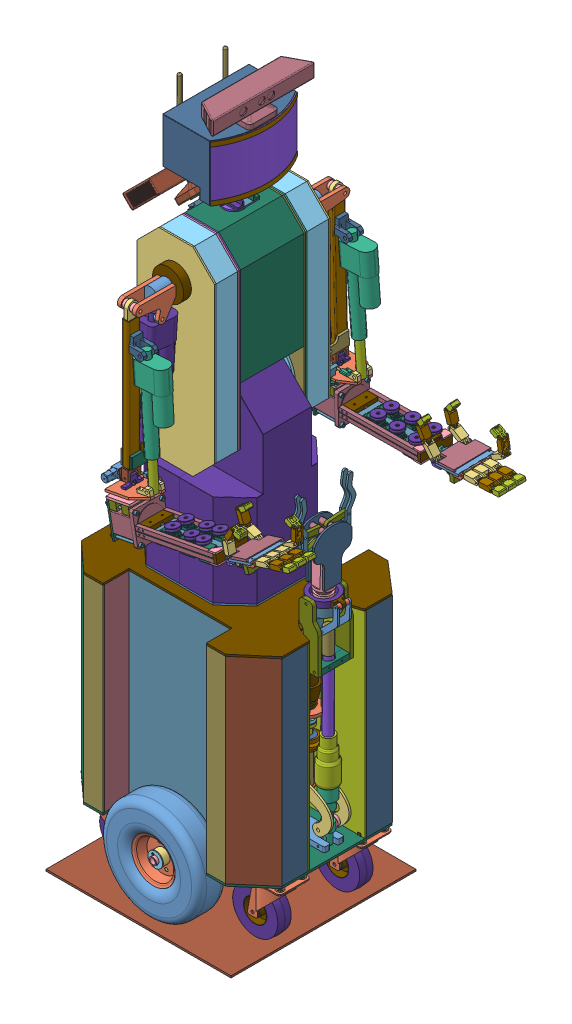
SolidWorks assembly sorbot, configuration По умолчанию. Lengths in mm.
Overall size (793.33 1880.98 665.85).
929 component instances, 299 part files, 1077 mates.
Components (placement in the parent):
- wheel-1: wheel [По умолчанию] at (-13.022 1.4469 17.7637) size (270 270 80)
  - wheel.chamber-1: wheel.chamber [По умолчанию] at (6.3301 10.4899 0) size (270 270 80)
  - wheel.metal.front-1: wheel.metal.front [По умолчанию] at (6.3301 10.4899 42.7077) x (-0.311346 0.950297 0) z (0.950297 0.311346 0) size (117.48 26.95 117.48)
  - wheel.metal.internal-1: wheel.metal.internal [По умолчанию] at (6.3301 10.4899 36.3681) x (0.950297 0.311346 0) z (-0.311346 0.950297 0) size (117.48 60 117.48)
- wheel-2: wheel [По умолчанию] at (1.0599 2.4489 -290) x (-0.989924 -0.141601 0) z (0 0 -1) size (270 270 80)
  - wheel.chamber-1: wheel.chamber [По умолчанию] at (6.3301 10.4899 0) size (270 270 80)
  - wheel.metal.front-1: wheel.metal.front [По умолчанию] at (6.3301 10.4899 42.7077) x (-0.311346 0.950297 0) z (0.950297 0.311346 0) size (117.48 26.95 117.48)
  - wheel.metal.internal-1: wheel.metal.internal [По умолчанию] at (6.3301 10.4899 36.3681) x (0.950297 0.311346 0) z (-0.311346 0.950297 0) size (117.48 60 117.48)
- wheel.axis-1: wheel.axis [По умолчанию] at (-6.6918 11.9368 88.1319) x (-0.923728 -0.383049 0) z (0 0 -1) size (20 20 450)
- wheel.washer-1: wheel.washer [По умолчанию] at (-6.6918 11.9368 79.1319) size (40 40 2)
- wheel.washer-2: wheel.washer [По умолчанию] at (-6.6918 11.9368 -353.3681) size (40 40 2)
- wheel.axis.splint-1: wheel.axis.splint [По умолчанию] at (-51.8409 -4.2239 -121.73) x (0.909121 0.380793 -0.168805) z (0.181229 0.003281 0.983435) size (4.99 27.52 1.94)
- wheel.axis.splint-2: wheel.axis.splint [По умолчанию] at (-119.6931 -47.4576 -189.7376) x (-0.699932 -0.282835 -0.65582) z (0.605814 0.251217 -0.754904) size (4.99 27.52 1.94)
- wheel.disk-1: wheel.disk [По умолчанию] at (-6.6918 11.9368 -326.3681) size (86 86 70)
- gearmotor-1: gearmotor [По умолчанию] at (53.2168 119.2767 -131.0001) x (0.993251 -0.115983 0) z (0 0 1) size (79 79 282)
- wheel.bearing-1: wheel.bearing [По умолчанию] at (-6.6918 11.9368 -263.3681) x (0.993854 -0.110698 0) z (0 0 1) size (32 32 7)
- wheel.stop.bearing-2: wheel.stop.bearing [По умолчанию] at (-3.289 9.2452 -250.3457) size (52.27 52.27 14.02)
  - wheel.stop.bearing.p1-1: wheel.stop.bearing.p1 [По умолчанию] at (-3.4029 2.6916 -6.0224) size (40 40 4)
  - wheel.stop.bearing.p2-1: wheel.stop.bearing.p2 [По умолчанию] at (-3.421 17.5634 1.5621) size (7 7 7)
  - wheel.stop.bearing.p1-2: wheel.stop.bearing.p1 [По умолчанию] at (-3.4029 2.6916 8) x (-0.923728 -0.383049 0) z (0 0 -1) size (40 40 4)
  - wheel.stop.bearing.p2-3: wheel.stop.bearing.p2 [По умолчанию] at (4.0173 15.58 1.5621) x (0.866025 -0.5 0) z (0 0 1) size (7 7 7)
  - wheel.stop.bearing.p2-4: wheel.stop.bearing.p2 [По умолчанию] at (9.4674 10.1432 1.5621) x (0.5 -0.866025 0) z (0 0 1) size (7 7 7)
  - wheel.stop.bearing.p2-5: wheel.stop.bearing.p2 [По умолчанию] at (11.469 2.7097 1.5621) x (0 -1 0) z (0 0 1) size (7 7 7)
  - wheel.stop.bearing.p2-6: wheel.stop.bearing.p2 [По умолчанию] at (9.4856 -4.7286 1.5621) x (-0.5 -0.866025 0) z (0 0 1) size (7 7 7)
  - wheel.stop.bearing.p2-7: wheel.stop.bearing.p2 [По умолчанию] at (4.0488 -10.1787 1.5621) x (-0.866025 -0.5 0) z (0 0 1) size (7 7 7)
  - wheel.stop.bearing.p2-8: wheel.stop.bearing.p2 [По умолчанию] at (-3.3847 -12.1802 1.5621) x (-1 0 0) z (0 0 1) size (7 7 7)
  - wheel.stop.bearing.p2-9: wheel.stop.bearing.p2 [По умолчанию] at (-10.8231 -10.1969 1.5621) x (-0.866025 0.5 0) z (0 0 1) size (7 7 7)
  - wheel.stop.bearing.p2-10: wheel.stop.bearing.p2 [По умолчанию] at (-16.2732 -4.76 1.5621) x (-0.5 0.866025 0) z (0 0 1) size (7 7 7)
  - wheel.stop.bearing.p2-11: wheel.stop.bearing.p2 [По умолчанию] at (-18.2747 2.6734 1.5621) x (0 1 0) z (0 0 1) size (7 7 7)
  - wheel.stop.bearing.p2-12: wheel.stop.bearing.p2 [По умолчанию] at (-16.2913 10.1118 1.5621) x (0.5 0.866025 0) z (0 0 1) size (7 7 7)
  - wheel.stop.bearing.p2-13: wheel.stop.bearing.p2 [По умолчанию] at (-10.8545 15.5619 1.5621) x (0.866025 0.5 0) z (0 0 1) size (7 7 7)
- sproket.initial-1: sproket.initial [По умолчанию] at (53.2168 119.2767 -271.5001) x (0.999977 0.00678 0) z (0 0 1) size (82.09 81.83 4.4)
- gearmotor.sprocket.wheel.disk-1: gearmotor.sprocket.wheel.disk [По умолчанию] at (53.2168 119.2767 -276.8747) x (0.999997 -0.002459 0) z (0 0 1) size (68 68 28.87)
- sprocket-1: sprocket [По умолчанию] at (-6.6918 11.9368 -271.3681) size (82.09 81.83 3)
- bottom-2: bottom [По умолчанию] at (-6.1674 46.4368 -211.0406) size (543.13 5.5 438.63)
- wheel.axis.frame-3: wheel.axis.frame [По умолчанию] at (43.3082 10.4368 -242.3457) x (-1 0 0) z (0 0 1) size (126 65.5 38)
- accumulator1-1: accumulator1 [По умолчанию] at (-171.7458 53.2126 -136.828) x (0 0 -1) z (1 0 0) size (232 218.1 175)
- wheel.disk-2: wheel.disk [По умолчанию] at (-6.6918 11.9368 54.1319) x (-0.923728 -0.383049 0) z (0 0 -1) size (86 86 70)
- wheel.bearing-2: wheel.bearing [По умолчанию] at (-6.6918 11.9368 -15.8681) size (32 32 7)
- wheel.stop.bearing-3: wheel.stop.bearing [По умолчанию] at (-3.289 9.2452 -23.8681) size (52.27 52.27 14.02)
  - wheel.stop.bearing.p1-1: wheel.stop.bearing.p1 [По умолчанию] at (-3.4029 2.6916 -6.0224) size (40 40 4)
  - wheel.stop.bearing.p2-1: wheel.stop.bearing.p2 [По умолчанию] at (-3.421 17.5634 1.5621) size (7 7 7)
  - wheel.stop.bearing.p1-2: wheel.stop.bearing.p1 [По умолчанию] at (-3.4029 2.6916 8) x (-0.923728 -0.383049 0) z (0 0 -1) size (40 40 4)
  - wheel.stop.bearing.p2-3: wheel.stop.bearing.p2 [По умолчанию] at (4.0173 15.58 1.5621) x (0.866025 -0.5 0) z (0 0 1) size (7 7 7)
  - wheel.stop.bearing.p2-4: wheel.stop.bearing.p2 [По умолчанию] at (9.4674 10.1432 1.5621) x (0.5 -0.866025 0) z (0 0 1) size (7 7 7)
  - wheel.stop.bearing.p2-5: wheel.stop.bearing.p2 [По умолчанию] at (11.469 2.7097 1.5621) x (0 -1 0) z (0 0 1) size (7 7 7)
  - wheel.stop.bearing.p2-6: wheel.stop.bearing.p2 [По умолчанию] at (9.4856 -4.7286 1.5621) x (-0.5 -0.866025 0) z (0 0 1) size (7 7 7)
  - wheel.stop.bearing.p2-7: wheel.stop.bearing.p2 [По умолчанию] at (4.0488 -10.1787 1.5621) x (-0.866025 -0.5 0) z (0 0 1) size (7 7 7)
  - wheel.stop.bearing.p2-8: wheel.stop.bearing.p2 [По умолчанию] at (-3.3847 -12.1802 1.5621) x (-1 0 0) z (0 0 1) size (7 7 7)
  - wheel.stop.bearing.p2-9: wheel.stop.bearing.p2 [По умолчанию] at (-10.8231 -10.1969 1.5621) x (-0.866025 0.5 0) z (0 0 1) size (7 7 7)
  - wheel.stop.bearing.p2-10: wheel.stop.bearing.p2 [По умолчанию] at (-16.2732 -4.76 1.5621) x (-0.5 0.866025 0) z (0 0 1) size (7 7 7)
  - wheel.stop.bearing.p2-11: wheel.stop.bearing.p2 [По умолчанию] at (-18.2747 2.6734 1.5621) x (0 1 0) z (0 0 1) size (7 7 7)
  - wheel.stop.bearing.p2-12: wheel.stop.bearing.p2 [По умолчанию] at (-16.2913 10.1118 1.5621) x (0.5 0.866025 0) z (0 0 1) size (7 7 7)
  - wheel.stop.bearing.p2-13: wheel.stop.bearing.p2 [По умолчанию] at (-10.8545 15.5619 1.5621) x (0.866025 0.5 0) z (0 0 1) size (7 7 7)
- wheel.axis.frame-4: wheel.axis.frame [По умолчанию] at (-56.6918 10.4368 -29.8906) x (1 0 0) z (0 0 -1) size (126 65.5 38)
- sprocket-2: sprocket [По умолчанию] at (-6.6918 11.9368 -3.8681) x (0.99994 0.010997 0) z (0 0 1) size (82.09 81.83 3)
- gearmotor-2: gearmotor [По умолчанию] at (-40.8776 119.0545 -142.1692) x (-0.999846 -0.017524 0) z (0 0 -1) size (79 79 282)
- gearmotor.sprocket.wheel.disk-2: gearmotor.sprocket.wheel.disk [По умолчанию] at (-40.8776 119.0545 3.7054) x (-0.999846 -0.017524 0) z (0 0 -1) size (68 68 28.87)
- sproket.initial-2: sproket.initial [По умолчанию] at (-40.8776 119.0545 -1.6692) x (-0.999994 -0.003421 0) z (0 0 -1) size (82.09 81.83 4.4)
- man1-2: man1 [По умолчанию] at (221.423 424.2117 -133.5351) x (0 0 -1) z (1 0 0) size (156.5 840.47 285.01)
  - man1.actuator-1: man1.actuator [По умолчанию] at (-0.3986 -205.8789 -139.5078) x (-1 0 0) z (0 1 0.000021) size (65 65 317.39)
    - man1.drive1-1: man1.drive1 [По умолчанию] at (-4.1866 0.6029 0) size (50 50 148.25)
    - man1.drive1.frame.p1-1: man1.drive1.frame.p1 [По умолчанию] at (-4.1866 0.6029 121) size (28 28 8)
    - man1.drive1.frame.p2-1: man1.drive1.frame.p2 [По умолчанию] at (-4.1866 0.6029 121) size (65 65 8)
    - man1.drive1.frame.p4-1: man1.drive1.frame.p4 [По умолчанию] at (-4.1866 0.6029 -33) size (54 65 20)
    - man1.drive1.frame.p5-1: man1.drive1.frame.p5 [По умолчанию] at (-4.1866 0.6029 -37.3912) x (0.999995 0.003021 0) z (0 0 1) size (41.77 41.77 245)
    - man1.drive1.frame.p6-1: man1.drive1.frame.p6 [По умолчанию] at (-4.1866 0.6029 129) size (30 30 25)
    - man1.drive1.frame.p7-1: man1.drive1.frame.p7 [По умолчанию] at (-4.1866 0.6029 154) size (30 30 2)
    - man1.drive1.frame.p8-1: man1.drive1.frame.p8 [По умолчанию] at (-4.1866 0.6029 156) size (30 30 28)
    - man1.drive1.frame.p10-1: man1.drive1.frame.p10 [По умолчанию] at (-4.1866 0.6029 164) size (10.5 10.5 116)
    - man1.drive1.frame.p9-1: man1.drive1.frame.p9 [По умолчанию] at (-4.1866 0.6029 187) size (65 65 28)
    - man1.drive1.frame.p11-1: man1.drive1.frame.p11 [По умолчанию] at (-4.1866 0.6029 187) size (35 35 24)
    - man1.drive1.frame.p3-7: man1.drive1.frame.p3 [По умолчанию] at (-4.1866 0.6029 58) (suppressed, hidden)
  - man1.p1-1: man1.p1 [По умолчанию] at (52.788 -228.8789 -138.9054) x (-1 0 0) z (0 0 1) size (100 8 8)
  - man1.drive1.frame.p12-1: man1.drive1.frame.p12 [По умолчанию] at (3.788 68.5641 -138.8992) x (-1 0 0) z (0 1 0.000021) size (21 21 93)
  - man1.p2-1: man1.p2 [По умолчанию] at (-22.212 -237.9208 -123.0814) x (0 0 -1) z (-1 0 0) size (72.27 30 90)
  - man1.p5-1: man1.p5 [По умолчанию] at (4.7507 160.9388 -85.9149) x (-1 0 0) z (0 -0.002225 0.999998) size (26 90 26)
  - man1.p4-1: man1.p4 [По умолчанию] at (3.7914 125.9389 -85.9928) x (0.93549 0.000786 -0.353351) z (-0.353352 0.002082 -0.935488) size (30 487 30)
  - man1.p3-2: man1.p3 [По умолчанию] at (38.7914 154.9807 -70.1243) x (0 0 -1) z (1 0 0) size (125.25 30 85)
  - man1.p6-1: man1.p6 [По умолчанию] at (42.008 145.9388 -85.9483) x (-1 0 0) z (0 0.364371 -0.931254) size (75 8 8)
  - man1.p7-2: man1.p7 [По умолчанию] at (23.8722 69.7096 -67.4428) x (-1 0 0) z (0 -0.002225 0.999998) size (74 91.83 135.45)
  - man1.actuator-2: man1.actuator [По умолчанию] at (8.0554 58.0922 -32.4461) x (1 0 0) z (0 -0.999998 -0.002148) size (65 65 317.39)
    - man1.drive1-1: man1.drive1 [По умолчанию] at (-4.1866 0.6029 0) size (50 50 148.25)
    - man1.drive1.frame.p1-1: man1.drive1.frame.p1 [По умолчанию] at (-4.1866 0.6029 121) size (28 28 8)
    - man1.drive1.frame.p2-1: man1.drive1.frame.p2 [По умолчанию] at (-4.1866 0.6029 121) size (65 65 8)
    - man1.drive1.frame.p4-1: man1.drive1.frame.p4 [По умолчанию] at (-4.1866 0.6029 -33) size (54 65 20)
    - man1.drive1.frame.p5-1: man1.drive1.frame.p5 [По умолчанию] at (-4.1866 0.6029 -37.3912) x (0.999995 0.003021 0) z (0 0 1) size (41.77 41.77 245)
    - man1.drive1.frame.p6-1: man1.drive1.frame.p6 [По умолчанию] at (-4.1866 0.6029 129) size (30 30 25)
    - man1.drive1.frame.p7-1: man1.drive1.frame.p7 [По умолчанию] at (-4.1866 0.6029 154) size (30 30 2)
    - man1.drive1.frame.p8-1: man1.drive1.frame.p8 [По умолчанию] at (-4.1866 0.6029 156) size (30 30 28)
    - man1.drive1.frame.p10-1: man1.drive1.frame.p10 [По умолчанию] at (-4.1866 0.6029 164) size (10.5 10.5 116)
    - man1.drive1.frame.p9-1: man1.drive1.frame.p9 [По умолчанию] at (-4.1866 0.6029 187) size (65 65 28)
    - man1.drive1.frame.p11-1: man1.drive1.frame.p11 [По умолчанию] at (-4.1866 0.6029 187) size (35 35 24)
    - man1.drive1.frame.p3-7: man1.drive1.frame.p3 [По умолчанию] at (-4.1866 0.6029 58) (suppressed, hidden)
  - man1.drive1.frame.p12-2: man1.drive1.frame.p12 [По умолчанию] at (3.8689 -153.2296 -32.2971) x (1 0 0) z (0 -0.999998 -0.002148) size (21 21 93)
  - man1.p8-1: man1.p8 [По умолчанию] at (3.7914 -359.7465 -87.0735) x (0 -0.002225 0.999998) z (-1 0 0) size (145 30 54.24)
  - man1.p11-2: man1.p11 [По умолчанию] at (-11.2086 -199.8321 18.3244) x (-1 0 0) z (0 0.071625 0.997432) size (5.5 105.72 90.08)
  - man1.p12-2: man1.p12 [По умолчанию] at (-22.7871 -224.5214 -51.2659) x (1 0 0) z (0 0.19273 0.981252) size (5.5 118.7 99.86)
  - man1.p13-1: man1.p13 [По умолчанию] at (-4.1311 -234.2294 -32.471) x (1 0 0) z (0 -0.069887 -0.997555) size (7 26 26)
  - man1.p13-2: man1.p13 [По умолчанию] at (-10.2871 -314.4644 20.4089) x (1 0 0) z (0 0 1) size (7 26 26)
  - man1.p13-3: man1.p13 [По умолчанию] at (18.8689 -234.2294 -32.471) size (7 26 26)
  - man1.p12-3: man1.p12 [По умолчанию] at (24.7129 -224.5214 -51.2659) x (1 0 0) z (0 0.19273 0.981252) size (5.5 118.7 99.86)
  - man1.p13-4: man1.p13 [По умолчанию] at (24.7129 -314.4644 20.4089) x (1 0 0) z (0 -0.270753 0.962649) size (7 26 26)
  - man1.drive2-1: man1.drive2 [По умолчанию] at (3.7079 -240.2809 21.0583) x (0.972815 -0.000504 0.231584) z (0 0.999998 0.002174) size (32 32 80.98)
  - man1.p14-1: man1.p14 [По умолчанию] at (3.7079 -243.1669 21.052) x (0.999283 0.000082 -0.03786) z (0.03786 -0.002173 0.999281) size (50 191 50)
  - man1.p15-1: man1.p15 [По умолчанию] at (3.7079 -218.9022 21.1047) x (0.998805 0.000106 -0.048869) z (0.048869 -0.002172 0.998803) size (52 118 52)
  - man1.p16-1: man1.p16 [По умолчанию] at (3.7079 -152.1041 21.25) x (0.992237 0.00027 -0.124359) z (0.12436 -0.002157 0.992235) size (24.7 240 24.7)
  - man1.p17-1: man1.p17 [По умолчанию] at (3.7079 -169.2808 21.2126) x (0.999945 0.000023 -0.010535) z (0.010535 -0.002174 0.999942) size (23 37 23)
  - man1.p18-1: man1.p18 [По умолчанию] at (3.7079 -154.5438 21.2447) x (0.916473 0.00087 -0.400097) z (0.400098 -0.001993 0.91647) size (10 240 10)
  - man1.stok.2-1: man1.stok.2 [По умолчанию] at (4.7586 68.5442 21.7351) x (0.999987 -0.000011 0.005102) z (-0.005102 -0.002174 0.999985) size (31.92 103 31.92)
    - man1.p19-1: man1.p19 [По умолчанию] at (-1.0508 -2.675 0) x (1 0 -0.000645) z (0.000645 0 1) size (14 6 15.86)
    - man1.p20-1: man1.p20 [По умолчанию] at (-1.0508 -12.2265 0) x (0.999987 0 -0.005102) z (0.005102 0 0.999987) size (24 100 24)
    - man1.p19-2: man1.p19 [По умолчанию] at (-1.0508 -9.0548 0) x (1 0 -0.000645) z (0.000645 0 1) size (14 6 15.86)
    - man1.p21-1: man1.p21 [По умолчанию] at (-1.0508 -8.2265 0) x (-0.905374 0 -0.424616) z (-0.424616 0 0.905374) size (24 7 24)
  - man1.drive3-1: man1.drive3 [По умолчанию] at (3.7079 189.134 9.0302) x (-0.018472 -0.002174 0.999827) z (-0.999829 0.00004 -0.018472) size (76 103.5 76)
  - man1.p22-1: man1.p22 [По умолчанию] at (3.7079 63.509 21.7188) x (0 -0.002174 0.999998) z (-1 0 0) size (20 15 76)
  - man1.p22-2: man1.p22 [По умолчанию] at (3.7079 63.509 21.7188) x (0 0.002174 -0.999998) z (1 0 0) size (20 15 76)
  - man1.p23-1: man1.p23 [По умолчанию] at (-44.2921 93.6528 21.7843) x (1 0 0) z (0 -0.002174 0.999998) size (10 166.6 51.35)
  - man1.p24-1: man1.p24 [По умолчанию] at (3.7079 212.1339 9.0802) x (1 0 0) z (0 -0.002174 0.999998) size (76 16 76)
  - man1.p25-1: man1.p25 [По умолчанию] at (3.7079 206.1339 9.0672) x (1 0 0) z (0 -0.002174 0.999998) size (30 16 20.8)
  - man1.p26-2: man1.p26 [По умолчанию] at (-14.0001 214.8868 58.3905) x (1 0 0) z (0 -0.797207 0.603707) size (5 86.81 49.56)
  - man1.p27-1: man1.p27 [По умолчанию] at (-11.2921 220.0261 58.6688) size (10 12 12)
  - man1.p23-2: man1.p23 [По умолчанию] at (41.7079 93.6528 21.7843) x (1 0 0) z (0 -0.002174 0.999998) size (10 166.6 51.35)
  - man1.p26-3: man1.p26 [По умолчанию] at (18.7079 214.8868 58.3905) x (1 0 0) z (0 -0.797207 0.603707) size (5 86.81 49.56)
  - man1.p27-2: man1.p27 [По умолчанию] at (8.7079 220.0261 58.6688) size (10 12 12)
  - man1.p28-1: man1.p28 [По умолчанию] at (3.7079 217.1339 9.0911) x (1 0 0) z (0 -0.002174 0.999998) size (44 5 44)
  - man1.p29-1: man1.p29 [По умолчанию] at (3.7079 222.1339 9.102) x (1 0 0) z (0 -0.002174 0.999998) size (48 87 48)
  - man1.drive4-2: man1.drive4 [По умолчанию] at (3.7079 240.9454 9.1429) x (1 0 0) z (0 0.999998 0.002174) size (32 32 76.8)
  - man1.p30-1: man1.p30 [По умолчанию] at (3.7079 323.4415 9.3222) x (1 0 0) z (0 -0.002174 0.999998) size (9 22 9.04)
  - man1.p31-1: man1.p31 [По умолчанию] at (29.5403 341.472 7.7592) x (-0.97166 0.236384 0.000514) z (0 -0.002174 0.999998) size (45 45 3.2)
  - man1.p32-1: man1.p32 [По умолчанию] at (3.7079 309.2075 9.2913) x (0.999646 0.000058 -0.02662) z (0.02662 -0.002173 0.999643) size (7 52 7)
  - man1.p31-2: man1.p31 [По умолчанию] at (-22.1256 341.472 7.7592) x (0.978079 0.208235 0.000453) z (0 -0.002174 0.999998) size (45 45 3.2)
  - man1.p33-1: man1.p33 [По умолчанию] at (3.7079 357.0484 9.3953) x (1 0 -0.000001) z (0.000001 -0.002174 0.999998) size (11 4 11)
  - man1.p34-1: man1.p34 [По умолчанию] at (3.917 277.9455 29.2556) x (1 0 0) z (0 -0.002174 0.999998) size (102 143.82 5)
  - man1.p35-1: man1.p35 [По умолчанию] at (3.5428 363.0979 -0.5593) x (1 0 0) z (0 -0.002174 0.999998) size (21.92 13.34 40.06)
  - man1.p34-2: man1.p34 [По умолчанию] at (3.9108 278.1144 -15.8086) x (1 0 0) z (0 -0.002174 0.999998) size (102 143.82 5)
  - man1.p36-1: man1.p36 [По умолчанию] at (-22.1256 341.7376 -114.3921) x (-0.911615 -0.411045 -0.000894) z (-0.411046 0.911612 0.001982) size (14 12.53 14)
  - man1.p36-4: man1.p36 [По умолчанию] at (29.5403 341.2593 105.5809) x (1 0 0) z (0 0.999998 0.002174) size (14 12.53 14)
  - man1.p36-5: man1.p36 [По умолчанию] at (-22.1256 341.6777 -86.858) x (0.923728 0.383048 0.000833) z (0.383049 -0.923726 -0.002008) size (14 12.53 14)
  - man1.p36-6: man1.p36 [По умолчанию] at (29.5403 341.6777 -86.8577) x (0.923728 0.383048 0.000833) z (0.383049 -0.923726 -0.002008) size (14 12.53 14)
  - man1.p39-1: man1.p39 [По умолчанию] at (-8.83 377.6785 -10.5921) x (1 0 0) z (0 -0.002174 0.999998) size (14 14 15)
  - man1.p39-2: man1.p39 [По умолчанию] at (-8.83 377.624 14.4723) x (-0.43245 -0.901656 -0.00196) z (0 -0.002174 0.999998) size (14 14 15)
  - man1.p40-1: man1.p40 [По умолчанию] at (-55.1239 334.4334 13.8439) x (0.999874 0.01586 0.000034) z (0 -0.002174 0.999998) size (24.21 150.81 5)
  - man1.p37-2: man1.p37 [По умолчанию] at (29.5403 341.4848 1.8592) x (-0.97166 0.236384 0.000514) z (0 -0.002174 0.999998) size (47.74 16 15)
  - man1.p37-3: man1.p37 [По умолчанию] at (-22.1256 341.4848 1.8592) x (0.978079 0.208235 0.000453) z (0 -0.002174 0.999998) size (47.74 16 15)
  - man1.p38-3: man1.p38 [По умолчанию] at (-20.7759 380.2262 4.9434) x (0.937414 -0.348215 -0.000757) z (0 -0.002174 0.999998) size (59.39 24.42 8)
  - man1.p40-5: man1.p40 [По умолчанию] at (-55.1239 334.4638 -0.1561) x (0.999874 0.01586 0.000034) z (0 -0.002174 0.999998) size (24.21 150.81 5)
  - man1.p39-5: man1.p39 [По умолчанию] at (15.9138 377.6793 -10.5921) x (1 0 0) z (0 -0.002174 0.999998) size (14 14 15)
  - man1.p40-6: man1.p40 [По умолчанию] at (62.3221 333.4728 18.8418) x (-0.999874 0.01586 0.000035) z (0 0.002174 -0.999998) size (24.21 150.81 5)
  - man1.p40-7: man1.p40 [По умолчанию] at (62.3221 333.5032 4.8418) x (-0.999874 0.01586 0.000035) z (0 0.002174 -0.999998) size (24.21 150.81 5)
  - man1.p38-4: man1.p38 [По умолчанию] at (28.1311 377.9713 4.9385) x (-0.993258 0.11592 0.000252) z (0 -0.002174 0.999998) size (59.39 24.42 8)
  - man1.p39-6: man1.p39 [По умолчанию] at (15.9138 377.6248 14.4723) x (1 0 0) z (0 -0.002174 0.999998) size (14 14 15)
  - man1.p11-4: man1.p11 [По умолчанию] at (18.7914 -373.8941 -100.5086) x (1 0 0) z (0 -0.955022 0.296534) size (5.5 105.72 90.08)
- gearmotor-3: gearmotor [По умолчанию] at (-20.0648 476.1505 -136.9555) x (1 0 0) z (0 -1 0) size (79 79 282)
- wheel1-1: wheel1 [По умолчанию] at (-196.5272 -62.2972 -25.6616) x (-1 0 0) z (0 0 -1) size (200.34 170.67 200.34)
  - wheel1.p1-1: wheel1.p1 [По умолчанию] at (-12.811 1.8421 0) size (125 125 36)
  - wheel1.p2-1: wheel1.p2 [По умолчанию] at (-12.811 1.8421 0.314) size (63.07 63.07 18)
  - wheel1.p2-2: wheel1.p2 [По умолчанию] at (-12.811 1.8421 -1.8658) x (-0.923728 -0.383049 0) z (0 0 -1) size (63.07 63.07 18)
  - wheel1.p3-1: wheel1.p3 [По умолчанию] at (-12.811 1.8421 -23.186) size (26 26 45)
  - wheel1.p4-1: wheel1.p4 [По умолчанию] at (24.859 90.4164 -1.436) size (105.01 101.57 85.69)
  - wheel1.p5-1: wheel1.p5 [По умолчанию] at (-14.7105 107.5716 -31.4713) x (-0.835986 -0.053146 -0.546171) z (-0.546944 0 0.837169) size (19.35 16 19.35)
  - wheel1.p5-2: wheel1.p5 [По умолчанию] at (64.4343 107.3349 28.3568) x (-0.998587 -0.053146 0) z (0 0 1) size (19.35 16 19.35)
  - wheel1.p5-3: wheel1.p5 [По умолчанию] at (64.0198 107.4544 -30.9637) x (-0.998587 -0.053146 0) z (0 0 1) size (19.35 16 19.35)
  - wheel1.p5-4: wheel1.p5 [По умолчанию] at (-14.3812 94.4397 28.6561) x (0.835986 0.053146 0.546171) z (-0.546944 0 0.837169) size (19.35 16 19.35)
- gearmotor.fixture.p3-1: gearmotor.fixture.p3 [По умолчанию] at (-40.8776 119.0545 -206.1702) x (0.994905 -0.100817 0) z (0 0 1) size (85.63 69.7 25)
- gearmotor.fixture.p2-3: gearmotor.fixture.p2 [По умолчанию] at (10.2084 53.4933 -65.0001) size (86 101.43 182)
- gearmotor.fixture.p3-2: gearmotor.fixture.p3 [По умолчанию] at (53.2274 119.174 -90.4218) x (0.994792 -0.101924 0) z (0 0 1) size (85.63 69.7 25)
- wheel1-5: wheel1 [По умолчанию] at (187.6309 -62.2985 -24.8952) size (200.34 170.67 200.34)
  - wheel1.p1-1: wheel1.p1 [По умолчанию] at (-12.811 1.8421 0) size (125 125 36)
  - wheel1.p2-1: wheel1.p2 [По умолчанию] at (-12.811 1.8421 0.314) size (63.07 63.07 18)
  - wheel1.p2-2: wheel1.p2 [По умолчанию] at (-12.811 1.8421 -1.8658) x (-0.923728 -0.383049 0) z (0 0 -1) size (63.07 63.07 18)
  - wheel1.p3-1: wheel1.p3 [По умолчанию] at (-12.811 1.8421 -23.186) size (26 26 45)
  - wheel1.p4-1: wheel1.p4 [По умолчанию] at (24.859 90.4164 -1.436) size (105.01 101.57 85.69)
  - wheel1.p5-1: wheel1.p5 [По умолчанию] at (-14.7105 107.5716 -31.4713) x (-0.835986 -0.053146 -0.546171) z (-0.546944 0 0.837169) size (19.35 16 19.35)
  - wheel1.p5-2: wheel1.p5 [По умолчанию] at (64.4343 107.3349 28.3568) x (-0.998587 -0.053146 0) z (0 0 1) size (19.35 16 19.35)
  - wheel1.p5-3: wheel1.p5 [По умолчанию] at (64.0198 107.4544 -30.9637) x (-0.998587 -0.053146 0) z (0 0 1) size (19.35 16 19.35)
  - wheel1.p5-4: wheel1.p5 [По умолчанию] at (-14.3812 94.4397 28.6561) x (0.835986 0.053146 0.546171) z (-0.546944 0 0.837169) size (19.35 16 19.35)
- wheel1-7: wheel1 [По умолчанию] at (-196.1639 -62.2105 -250.4568) x (-1 0 0) z (0 0 -1) size (200.34 170.67 200.34)
  - wheel1.p1-1: wheel1.p1 [По умолчанию] at (-12.811 1.8421 0) size (125 125 36)
  - wheel1.p2-1: wheel1.p2 [По умолчанию] at (-12.811 1.8421 0.314) size (63.07 63.07 18)
  - wheel1.p2-2: wheel1.p2 [По умолчанию] at (-12.811 1.8421 -1.8658) x (-0.923728 -0.383049 0) z (0 0 -1) size (63.07 63.07 18)
  - wheel1.p3-1: wheel1.p3 [По умолчанию] at (-12.811 1.8421 -23.186) size (26 26 45)
  - wheel1.p4-1: wheel1.p4 [По умолчанию] at (24.859 90.4164 -1.436) size (105.01 101.57 85.69)
  - wheel1.p5-1: wheel1.p5 [По умолчанию] at (-14.7105 107.5716 -31.4713) x (-0.835986 -0.053146 -0.546171) z (-0.546944 0 0.837169) size (19.35 16 19.35)
  - wheel1.p5-2: wheel1.p5 [По умолчанию] at (64.4343 107.3349 28.3568) x (-0.998587 -0.053146 0) z (0 0 1) size (19.35 16 19.35)
  - wheel1.p5-3: wheel1.p5 [По умолчанию] at (64.0198 107.4544 -30.9637) x (-0.998587 -0.053146 0) z (0 0 1) size (19.35 16 19.35)
  - wheel1.p5-4: wheel1.p5 [По умолчанию] at (-14.3812 94.4397 28.6561) x (0.835986 0.053146 0.546171) z (-0.546944 0 0.837169) size (19.35 16 19.35)
- wheel1-8: wheel1 [По умолчанию] at (187.4476 -61.9053 -246.5204) size (200.34 170.67 200.34)
  - wheel1.p1-1: wheel1.p1 [По умолчанию] at (-12.811 1.8421 0) size (125 125 36)
  - wheel1.p2-1: wheel1.p2 [По умолчанию] at (-12.811 1.8421 0.314) size (63.07 63.07 18)
  - wheel1.p2-2: wheel1.p2 [По умолчанию] at (-12.811 1.8421 -1.8658) x (-0.923728 -0.383049 0) z (0 0 -1) size (63.07 63.07 18)
  - wheel1.p3-1: wheel1.p3 [По умолчанию] at (-12.811 1.8421 -23.186) size (26 26 45)
  - wheel1.p4-1: wheel1.p4 [По умолчанию] at (24.859 90.4164 -1.436) size (105.01 101.57 85.69)
  - wheel1.p5-1: wheel1.p5 [По умолчанию] at (-14.7105 107.5716 -31.4713) x (-0.835986 -0.053146 -0.546171) z (-0.546944 0 0.837169) size (19.35 16 19.35)
  - wheel1.p5-2: wheel1.p5 [По умолчанию] at (64.4343 107.3349 28.3568) x (-0.998587 -0.053146 0) z (0 0 1) size (19.35 16 19.35)
  - wheel1.p5-3: wheel1.p5 [По умолчанию] at (64.0198 107.4544 -30.9637) x (-0.998587 -0.053146 0) z (0 0 1) size (19.35 16 19.35)
  - wheel1.p5-4: wheel1.p5 [По умолчанию] at (-14.3812 94.4397 28.6561) x (0.835986 0.053146 0.546171) z (-0.546944 0 0.837169) size (19.35 16 19.35)
- wall1-1: wall1 [По умолчанию] at (26.1889 166.4368 -212.2424) x (0 0 1) z (-1 0 0) size (150 418.71 5)
- wall2-1: wall2 [По умолчанию] at (21.1889 166.4368 -62.2424) size (245.99 533.21 4)
- wall2-2: wall2 [По умолчанию] at (21.1889 166.4368 -216.2424) size (245.99 533.21 4)
- wall3-1: wall3 [По умолчанию] at (57.626 166.4368 -212.2424) x (0 0 1) z (-1 0 0) size (150 5 80.99)
- wall4-1: wall4 [По умолчанию] at (102.1741 112.2872 -162.1841) size (5 115 160)
- wall6-1: wall6 [По умолчанию] at (262.1742 51.9368 -58.2424) size (4 533.21 70.07)
- wall7-1: wall7 [По умолчанию] at (263.5274 51.9368 8.4769) x (0.650583 0 0.759435) z (-0.759435 0 0.650583) size (4 533.21 108.33)
- wall6-3: wall6 [По умолчанию] at (262.1742 585.1505 -216.2424) x (1 0 0) z (0 0 -1) size (4 533.21 70.07)
- wall7-3: wall7 [По умолчанию] at (182.0437 51.9368 -352.0328) x (0.650583 0 -0.759435) z (0.759435 0 0.650583) size (4 533.21 108.33)
- wall8-1: wall8 [По умолчанию] at (132.9009 51.9368 77.4522) size (52.1 533.21 4)
- wall8-2: wall8 [По умолчанию] at (132.798 585.1505 -351.1821) x (1 0 0) z (0 0 -1) size (52.1 533.21 4)
- wall9-1: wall9 [По умолчанию] at (131.9009 51.9368 18.6982) size (4 533.21 69.9)
- wall10-1: wall10 [По умолчанию] at (-1.8874 51.9368 6.1109) size (279.58 533.21 4)
- wall9-2: wall9 [По умолчанию] at (-151.6756 51.9368 18.7781) size (4 533.21 69.9)
- wall8-4: wall8 [По умолчанию] at (-146.6756 585.1505 77.4522) x (-1 0 0) z (0 0 1) size (52.1 533.21 4)
- wall7-v1-1: wall7-v1 [По умолчанию] at (-275.291 585.1505 5.6816) x (-0.67421 0 0.73854) z (0.73854 0 0.67421) size (4 533.21 104.08)
- wall11-1: wall11 [По умолчанию] at (-275.9003 51.4368 11.9312) size (4 556.08 297.39)
- wall7-v1-2: wall7-v1 [По умолчанию] at (-192.6496 585.1505 -354.9488) x (-0.67421 0 -0.73854) z (-0.73854 0 0.67421) size (4 533.21 104.08)
- wall8-5: wall8 [По умолчанию] at (-146.715 51.9368 -351.1236) x (-1 0 0) z (0 0 -1) size (52.1 533.21 4)
- wall9-3: wall9 [По умолчанию] at (-151.8245 51.9368 -341.8827) size (4 533.21 69.9)
- wall10-v1-1: wall10-v1 [По умолчанию] at (-12.0361 51.9368 -280.7872) x (-1 0 0) z (0 0 -1) size (279.58 533.21 4)
- wall9-4: wall9 [По умолчанию] at (131.7521 51.9368 -341.8827) size (4 533.21 69.9)
- cap-1: cap [По умолчанию] at (-5.7427 585.1505 -210.9644) x (0.999999 0 0.001245) z (-0.001245 0 0.999999) size (543.13 5 438.63)
- wall-fixture-v1-1: wall-fixture-v1 [По умолчанию] at (-173.7475 76.9368 76.4353) x (0 0 -1) z (1 0 0) size (22 468 22)
- wall-fixture-v2-1: wall-fixture-v2 [По умолчанию] at (-193.3747 76.9368 76.9391) size (36.03 468.21 15.37)
- wall-fixture-v2-1-1: wall-fixture-v2-1 [По умолчанию] at (-267.8225 76.9368 11.8405) x (0.73854 0 0.67421) z (-0.67421 0 0.73854) size (35.21 468.21 16.9)
- wall-fixture-v1-2: wall-fixture-v1 [По умолчанию] at (-129.6037 76.9368 8.4522) x (0 0 1) z (-1 0 0) size (22 468 22)
- wall-fixture-v2-1-2: wall-fixture-v2-1 [По умолчанию] at (-270.3872 51.4368 -279.8709) x (0 0 1) z (-1 0 0) size (35.21 468.21 16.9)
- wall-fixture-v2-2: wall-fixture-v2 [По умолчанию] at (-198.9245 51.4368 -348.5071) x (-0.738029 0 0.674769) z (-0.674769 0 -0.738029) size (36.03 468.21 15.37)
- wall-fixture-v1-3: wall-fixture-v1 [По умолчанию] at (-152.8245 51.4368 -329.0518) x (-1 0 0) z (0 0 -1) size (22 468 22)
- wall-fixture-v1-4: wall-fixture-v1 [По умолчанию] at (-150.8245 51.4368 -303.2005) size (22 468 22)
- wall-fixture-v1-5: wall-fixture-v1 [По умолчанию] at (115.6802 51.4368 -282.1286) x (0 0 -1) z (1 0 0) size (22 468 22)
- wall-fixture-v1-6: wall-fixture-v1 [По умолчанию] at (159.8239 51.4368 -350.1821) x (0 0 1) z (-1 0 0) size (22 468 22)
- wall-fixture-v2-2-1: wall-fixture-v2-2 [По умолчанию] at (179.7171 51.4368 -350.669) x (-1 0 0) z (0 0 -1) size (37.63 460 15.83)
- wall-fixture-v2-3-1: wall-fixture-v2-3 [По умолчанию] at (259.0363 51.4368 -285.4128) x (-0.759435 0 -0.650583) z (0.650583 0 -0.759435) size (34.89 460 17.21)
- wall-fixture-v1-7: wall-fixture-v1 [По умолчанию] at (240.1022 51.4368 -218.2424) x (0 0 -1) z (1 0 0) size (22 468 22)
- wall-fixture-v1-8: wall-fixture-v1 [По умолчанию] at (261.1742 51.4368 -35.1705) x (-1 0 0) z (0 0 -1) size (22 468 22)
- wall-fixture-v2-4-1: wall-fixture-v2-4 [По умолчанию] at (259.1218 591.4368 11.3719) x (-0.758224 0 0.651995) z (0.651995 0 0.758224) size (34.89 460 17.21)
- wall-fixture-v2-5-1: wall-fixture-v2-5 [По умолчанию] at (178.2705 591.4368 76.9391) x (-1 0 0) z (0 0 1) size (37.63 460 15.83)
- wall-fixture-v1-9: wall-fixture-v1 [По умолчанию] at (138.9009 51.4368 55.3804) size (22 468 22)
- wall-fixture-v1-10: wall-fixture-v1 [По умолчанию] at (136.9009 76.9368 29.5241) x (-1 0 0) z (0 0 -1) size (22 468 22)
- wall-fixture-6-1: wall-fixture-6 [По умолчанию] at (79.1022 164.4368 -79.0844) x (0 -1 0) z (1 0 0) size (22 116 22)
- wall-fixture-6-2: wall-fixture-6 [По умолчанию] at (21.1889 187.5087 -195.3202) x (1 0 0) z (0 -1 0) size (22 116 22)
- wall-fixture-7-1: wall-fixture-7 [По умолчанию] at (21.2432 187.5087 -58.2424) x (0 0 -1) z (0 -1 0) size (22 81 22)
- wall-fixture-7-2: wall-fixture-7 [По умолчанию] at (102.2155 187.5087 -216.2424) x (0 0 1) z (0 -1 0) size (22 81 22)
- wall-fixture-8-1: wall-fixture-8 [По умолчанию] at (123.2459 51.3998 -216.2424) x (0 0 1) z (-1 0 0) size (22 112 22)
- wall-fixture-8-2: wall-fixture-8 [По умолчанию] at (102.1741 51.9112 -79.3142) size (22 112 22)
- wall-fixture-9-1: wall-fixture-9 [По умолчанию] at (21.1889 187.3953 -79.3142) size (22 390 22)
- wall-fixture-9-2: wall-fixture-9 [По умолчанию] at (42.2608 187.5289 -216.2424) x (0 0 1) z (-1 0 0) size (22 390 22)
- turret-1: turret [По умолчанию] at (-28.0267 628.2367 -136.0551) x (0.993667 0 -0.112365) z (0.112365 0 0.993667) size (200 17.64 200)
  - turret-p1-1: turret-p1 [По умолчанию] at (8.0127 -33.0433 0) size (180 12.6 180)
  - turret-p2-1: turret-p2 [По умолчанию] at (70.5799 -32.9814 -33.6477) size (10 10 10)
  - turret-p2-2: turret-p2 [По умолчанию] at (54.1999 -32.9814 -53.9774) x (0.932472 0 -0.361242) z (0.361242 0 0.932472) size (10 10 10)
  - turret-p2-3: turret-p2 [По умолчанию] at (31.5821 -32.9814 -67.0172) x (0.739009 0 -0.673696) z (0.673696 0 0.739009) size (10 10 10)
  - turret-p2-4: turret-p2 [По умолчанию] at (5.7811 -32.9814 -71.0059) x (0.445738 0 -0.895163) z (0.895163 0 0.445738) size (10 10 10)
  - turret-p2-5: turret-p2 [По умолчанию] at (-19.7185 -32.9814 -65.4049) x (0.092268 0 -0.995734) z (0.995734 0 0.092268) size (10 10 10)
  - turret-p2-6: turret-p2 [По умолчанию] at (-41.4728 -32.9814 -50.9706) x (-0.273663 0 -0.961826) z (0.961826 0 -0.273663) size (10 10 10)
  - turret-p2-7: turret-p2 [По умолчанию] at (-56.5439 -32.9814 -29.6524) x (-0.602635 0 -0.798017) z (0.798017 0 -0.602635) size (10 10 10)
  - turret-p2-8: turret-p2 [По умолчанию] at (-62.8962 -32.9814 -4.3296) x (-0.850217 0 -0.526432) z (0.526432 0 -0.850217) size (10 10 10)
  - turret-p2-9: turret-p2 [По умолчанию] at (-59.6719 -32.9814 21.5781) x (-0.982973 0 -0.18375) z (0.18375 0 -0.982973) size (10 10 10)
  - turret-p2-10: turret-p2 [По умолчанию] at (-47.3064 -32.9814 44.5714) x (-0.982973 0 0.18375) z (-0.18375 0 -0.982973) size (10 10 10)
  - turret-p2-11: turret-p2 [По умолчанию] at (-27.4698 -32.9814 61.5452) x (-0.850217 0 0.526432) z (-0.526432 0 -0.850217) size (10 10 10)
  - turret-p2-12: turret-p2 [По умолчанию] at (-2.8411 -32.9814 70.2069) x (-0.602635 0 0.798017) z (-0.798017 0 -0.602635) size (10 10 10)
  - turret-p2-13: turret-p2 [По умолчанию] at (23.2535 -32.9814 69.3868) x (-0.273663 0 0.961826) z (-0.961826 0 -0.273663) size (10 10 10)
  - turret-p2-14: turret-p2 [По умолчанию] at (47.2898 -32.9814 59.1957) x (0.092268 0 0.995734) z (-0.995734 0 0.092268) size (10 10 10)
  - turret-p2-15: turret-p2 [По умолчанию] at (66.0214 -32.9814 41.0098) x (0.445738 0 0.895163) z (-0.895163 0 0.445738) size (10 10 10)
  - turret-p2-16: turret-p2 [По умолчанию] at (76.9187 -32.9814 17.2853) x (0.739009 0 0.673696) z (-0.673696 0 0.739009) size (10 10 10)
  - turret-p2-17: turret-p2 [По умолчанию] at (78.5098 -32.9814 -8.7736) x (0.932472 0 0.361242) z (-0.361242 0 0.932472) size (10 10 10)
  - turret-p3-1: turret-p3 [По умолчанию] at (8.0127 -35.0433 0) x (0.999999 0 0.001108) z (-0.001108 0 0.999999) size (180 2 180)
  - turret-p5-1: turret-p5 [По умолчанию] at (92.4476 -23.6726 -1.2982) size (3 3 3)
  - turret-p5-2: turret-p5 [По умолчанию] at (92.1994 -23.6726 -6.5974) x (0.998027 0 -0.062791) z (0.062791 0 0.998027) size (3 3 3)
  - turret-p5-3: turret-p5 [По умолчанию] at (91.6191 -23.6726 -11.8705) x (0.992115 0 -0.125333) z (0.125333 0 0.992115) size (3 3 3)
  - turret-p5-4: turret-p5 [По умолчанию] at (90.7087 -23.6726 -17.0968) x (0.982287 0 -0.187381) z (0.187381 0 0.982287) size (3 3 3)
  - turret-p5-5: turret-p5 [По умолчанию] at (89.472 -23.6726 -22.2556) x (0.968583 0 -0.24869) z (0.24869 0 0.968583) size (3 3 3)
  - turret-p5-6: turret-p5 [По умолчанию] at (87.9138 -23.6726 -27.3265) x (0.951057 0 -0.309017) z (0.309017 0 0.951057) size (3 3 3)
  - turret-p5-7: turret-p5 [По умолчанию] at (86.0403 -23.6726 -32.2896) x (0.929776 0 -0.368125) z (0.368125 0 0.929776) size (3 3 3)
  - turret-p5-8: turret-p5 [По умолчанию] at (83.8589 -23.6726 -37.1253) x (0.904827 0 -0.425779) z (0.425779 0 0.904827) size (3 3 3)
  - turret-p5-9: turret-p5 [По умолчанию] at (81.3781 -23.6726 -41.8145) x (0.876307 0 -0.481754) z (0.481754 0 0.876307) size (3 3 3)
  - turret-p5-10: turret-p5 [По умолчанию] at (78.6078 -23.6726 -46.3386) x (0.844328 0 -0.535827) z (0.535827 0 0.844328) size (3 3 3)
  - turret-p5-11: turret-p5 [По умолчанию] at (75.5589 -23.6726 -50.6799) x (0.809017 0 -0.587785) z (0.587785 0 0.809017) size (3 3 3)
  - turret-p5-12: turret-p5 [По умолчанию] at (72.2433 -23.6726 -54.8211) x (0.770513 0 -0.637424) z (0.637424 0 0.770513) size (3 3 3)
  - turret-p5-13: turret-p5 [По умолчанию] at (68.6744 -23.6726 -58.746) x (0.728969 0 -0.684547) z (0.684547 0 0.728969) size (3 3 3)
  - turret-p5-14: turret-p5 [По умолчанию] at (64.866 -23.6726 -62.4391) x (0.684547 0 -0.728969) z (0.728969 0 0.684547) size (3 3 3)
  - turret-p5-15: turret-p5 [По умолчанию] at (60.8332 -23.6726 -65.8857) x (0.637424 0 -0.770513) z (0.770513 0 0.637424) size (3 3 3)
  - turret-p5-16: turret-p5 [По умолчанию] at (56.592 -23.6726 -69.0723) x (0.587785 0 -0.809017) z (0.809017 0 0.587785) size (3 3 3)
  - turret-p5-17: turret-p5 [По умолчанию] at (52.159 -23.6726 -71.9864) x (0.535827 0 -0.844328) z (0.844328 0 0.535827) size (3 3 3)
  - turret-p5-18: turret-p5 [По умолчанию] at (47.5518 -23.6726 -74.6163) x (0.481754 0 -0.876307) z (0.876307 0 0.481754) size (3 3 3)
  - turret-p5-19: turret-p5 [По умолчанию] at (42.7886 -23.6726 -76.9517) x (0.425779 0 -0.904827) z (0.904827 0 0.425779) size (3 3 3)
  - turret-p5-20: turret-p5 [По умолчанию] at (37.8882 -23.6726 -78.9835) x (0.368125 0 -0.929776) z (0.929776 0 0.368125) size (3 3 3)
  - turret-p5-21: turret-p5 [По умолчанию] at (32.8698 -23.6726 -80.7035) x (0.309017 0 -0.951057) z (0.951057 0 0.309017) size (3 3 3)
  - turret-p5-22: turret-p5 [По умолчанию] at (27.7533 -23.6726 -82.1051) x (0.24869 0 -0.968583) z (0.968583 0 0.24869) size (3 3 3)
  - turret-p5-23: turret-p5 [По умолчанию] at (22.559 -23.6726 -83.1826) x (0.187381 0 -0.982287) z (0.982287 0 0.187381) size (3 3 3)
  - turret-p5-24: turret-p5 [По умолчанию] at (17.3072 -23.6726 -83.9318) x (0.125333 0 -0.992115) z (0.992115 0 0.125333) size (3 3 3)
  - turret-p5-25: turret-p5 [По умолчанию] at (12.0187 -23.6726 -84.3498) x (0.062791 0 -0.998027) z (0.998027 0 0.062791) size (3 3 3)
  - turret-p5-26: turret-p5 [По умолчанию] at (6.7144 -23.6726 -84.4349) x (0 0 -1) z (1 0 0) size (3 3 3)
  - turret-p5-27: turret-p5 [По умолчанию] at (1.4153 -23.6726 -84.1868) x (-0.062791 0 -0.998027) z (0.998027 0 -0.062791) size (3 3 3)
  - turret-p5-28: turret-p5 [По умолчанию] at (-3.8578 -23.6726 -83.6064) x (-0.125333 0 -0.992115) z (0.992115 0 -0.125333) size (3 3 3)
  - turret-p5-29: turret-p5 [По умолчанию] at (-9.0841 -23.6726 -82.696) x (-0.187381 0 -0.982287) z (0.982287 0 -0.187381) size (3 3 3)
  - turret-p5-30: turret-p5 [По умолчанию] at (-14.2429 -23.6726 -81.4594) x (-0.24869 0 -0.968583) z (0.968583 0 -0.24869) size (3 3 3)
  - turret-p5-31: turret-p5 [По умолчанию] at (-19.3138 -23.6726 -79.9012) x (-0.309017 0 -0.951057) z (0.951057 0 -0.309017) size (3 3 3)
  - turret-p5-32: turret-p5 [По умолчанию] at (-24.2769 -23.6726 -78.0277) x (-0.368125 0 -0.929776) z (0.929776 0 -0.368125) size (3 3 3)
  - turret-p5-33: turret-p5 [По умолчанию] at (-29.1126 -23.6726 -75.8462) x (-0.425779 0 -0.904827) z (0.904827 0 -0.425779) size (3 3 3)
  - turret-p5-34: turret-p5 [По умолчанию] at (-33.8018 -23.6726 -73.3654) x (-0.481754 0 -0.876307) z (0.876307 0 -0.481754) size (3 3 3)
  - turret-p5-35: turret-p5 [По умолчанию] at (-38.3259 -23.6726 -70.5951) x (-0.535827 0 -0.844328) z (0.844328 0 -0.535827) size (3 3 3)
  - turret-p5-36: turret-p5 [По умолчанию] at (-42.6672 -23.6726 -67.5462) x (-0.587785 0 -0.809017) z (0.809017 0 -0.587785) size (3 3 3)
  - turret-p5-37: turret-p5 [По умолчанию] at (-46.8085 -23.6726 -64.2307) x (-0.637424 0 -0.770513) z (0.770513 0 -0.637424) size (3 3 3)
  - turret-p5-38: turret-p5 [По умолчанию] at (-50.7334 -23.6726 -60.6617) x (-0.684547 0 -0.728969) z (0.728969 0 -0.684547) size (3 3 3)
  - turret-p5-39: turret-p5 [По умолчанию] at (-54.4264 -23.6726 -56.8533) x (-0.728969 0 -0.684547) z (0.684547 0 -0.728969) size (3 3 3)
  - turret-p5-40: turret-p5 [По умолчанию] at (-57.873 -23.6726 -52.8205) x (-0.770513 0 -0.637424) z (0.637424 0 -0.770513) size (3 3 3)
  - turret-p5-41: turret-p5 [По умолчанию] at (-61.0597 -23.6726 -48.5793) x (-0.809017 0 -0.587785) z (0.587785 0 -0.809017) size (3 3 3)
  - turret-p5-42: turret-p5 [По умолчанию] at (-63.9737 -23.6726 -44.1463) x (-0.844328 0 -0.535827) z (0.535827 0 -0.844328) size (3 3 3)
  - turret-p5-43: turret-p5 [По умолчанию] at (-66.6036 -23.6726 -39.5392) x (-0.876307 0 -0.481754) z (0.481754 0 -0.876307) size (3 3 3)
  - turret-p5-44: turret-p5 [По умолчанию] at (-68.9391 -23.6726 -34.7759) x (-0.904827 0 -0.425779) z (0.425779 0 -0.904827) size (3 3 3)
  - turret-p5-45: turret-p5 [По умолчанию] at (-70.9708 -23.6726 -29.8755) x (-0.929776 0 -0.368125) z (0.368125 0 -0.929776) size (3 3 3)
  - turret-p5-46: turret-p5 [По умолчанию] at (-72.6908 -23.6726 -24.8571) x (-0.951057 0 -0.309017) z (0.309017 0 -0.951057) size (3 3 3)
  - turret-p5-47: turret-p5 [По умолчанию] at (-74.0924 -23.6726 -19.7407) x (-0.968583 0 -0.24869) z (0.24869 0 -0.968583) size (3 3 3)
  - turret-p5-48: turret-p5 [По умолчанию] at (-75.1699 -23.6726 -14.5463) x (-0.982287 0 -0.187381) z (0.187381 0 -0.982287) size (3 3 3)
  - turret-p5-49: turret-p5 [По умолчанию] at (-75.9191 -23.6726 -9.2945) x (-0.992115 0 -0.125333) z (0.125333 0 -0.992115) size (3 3 3)
  - turret-p5-50: turret-p5 [По умолчанию] at (-76.3371 -23.6726 -4.006) x (-0.998027 0 -0.062791) z (0.062791 0 -0.998027) size (3 3 3)
  - turret-p5-51: turret-p5 [По умолчанию] at (-76.4222 -23.6726 1.2982) x (-1 0 0) z (0 0 -1) size (3 3 3)
  - turret-p5-52: turret-p5 [По умолчанию] at (-76.1741 -23.6726 6.5974) x (-0.998027 0 0.062791) z (-0.062791 0 -0.998027) size (3 3 3)
  - turret-p5-53: turret-p5 [По умолчанию] at (-75.5937 -23.6726 11.8705) x (-0.992115 0 0.125333) z (-0.125333 0 -0.992115) size (3 3 3)
  - turret-p5-54: turret-p5 [По умолчанию] at (-74.6834 -23.6726 17.0968) x (-0.982287 0 0.187381) z (-0.187381 0 -0.982287) size (3 3 3)
  - turret-p5-55: turret-p5 [По умолчанию] at (-73.4467 -23.6726 22.2556) x (-0.968583 0 0.24869) z (-0.24869 0 -0.968583) size (3 3 3)
  - turret-p5-56: turret-p5 [По умолчанию] at (-71.8885 -23.6726 27.3265) x (-0.951057 0 0.309017) z (-0.309017 0 -0.951057) size (3 3 3)
  - turret-p5-57: turret-p5 [По умолчанию] at (-70.015 -23.6726 32.2896) x (-0.929776 0 0.368125) z (-0.368125 0 -0.929776) size (3 3 3)
  - turret-p5-58: turret-p5 [По умолчанию] at (-67.8335 -23.6726 37.1253) x (-0.904827 0 0.425779) z (-0.425779 0 -0.904827) size (3 3 3)
  - turret-p5-59: turret-p5 [По умолчанию] at (-65.3527 -23.6726 41.8145) x (-0.876307 0 0.481754) z (-0.481754 0 -0.876307) size (3 3 3)
  - turret-p5-60: turret-p5 [По умолчанию] at (-62.5824 -23.6726 46.3386) x (-0.844328 0 0.535827) z (-0.535827 0 -0.844328) size (3 3 3)
  - turret-p5-61: turret-p5 [По умолчанию] at (-59.5335 -23.6726 50.6799) x (-0.809017 0 0.587785) z (-0.587785 0 -0.809017) size (3 3 3)
  - turret-p5-62: turret-p5 [По умолчанию] at (-56.218 -23.6726 54.8211) x (-0.770513 0 0.637424) z (-0.637424 0 -0.770513) size (3 3 3)
  - turret-p5-63: turret-p5 [По умолчанию] at (-52.649 -23.6726 58.746) x (-0.728969 0 0.684547) z (-0.684547 0 -0.728969) size (3 3 3)
  - turret-p5-64: turret-p5 [По умолчанию] at (-48.8406 -23.6726 62.4391) x (-0.684547 0 0.728969) z (-0.728969 0 -0.684547) size (3 3 3)
  - turret-p5-65: turret-p5 [По умолчанию] at (-44.8078 -23.6726 65.8857) x (-0.637424 0 0.770513) z (-0.770513 0 -0.637424) size (3 3 3)
  - turret-p5-66: turret-p5 [По умолчанию] at (-40.5666 -23.6726 69.0723) x (-0.587785 0 0.809017) z (-0.809017 0 -0.587785) size (3 3 3)
  - turret-p5-67: turret-p5 [По умолчанию] at (-36.1337 -23.6726 71.9864) x (-0.535827 0 0.844328) z (-0.844328 0 -0.535827) size (3 3 3)
  - turret-p5-68: turret-p5 [По умолчанию] at (-31.5265 -23.6726 74.6163) x (-0.481754 0 0.876307) z (-0.876307 0 -0.481754) size (3 3 3)
  - turret-p5-69: turret-p5 [По умолчанию] at (-26.7633 -23.6726 76.9517) x (-0.425779 0 0.904827) z (-0.904827 0 -0.425779) size (3 3 3)
  - turret-p5-70: turret-p5 [По умолчанию] at (-21.8628 -23.6726 78.9835) x (-0.368125 0 0.929776) z (-0.929776 0 -0.368125) size (3 3 3)
  - turret-p5-71: turret-p5 [По умолчанию] at (-16.8444 -23.6726 80.7035) x (-0.309017 0 0.951057) z (-0.951057 0 -0.309017) size (3 3 3)
  - turret-p5-72: turret-p5 [По умолчанию] at (-11.728 -23.6726 82.1051) x (-0.24869 0 0.968583) z (-0.968583 0 -0.24869) size (3 3 3)
  - turret-p5-73: turret-p5 [По умолчанию] at (-6.5336 -23.6726 83.1826) x (-0.187381 0 0.982287) z (-0.982287 0 -0.187381) size (3 3 3)
  - turret-p5-74: turret-p5 [По умолчанию] at (-1.2818 -23.6726 83.9318) x (-0.125333 0 0.992115) z (-0.992115 0 -0.125333) size (3 3 3)
  - turret-p5-75: turret-p5 [По умолчанию] at (4.0066 -23.6726 84.3498) x (-0.062791 0 0.998027) z (-0.998027 0 -0.062791) size (3 3 3)
  - turret-p5-76: turret-p5 [По умолчанию] at (9.3109 -23.6726 84.4349) x (0 0 1) z (-1 0 0) size (3 3 3)
  - turret-p5-77: turret-p5 [По умолчанию] at (14.6101 -23.6726 84.1868) x (0.062791 0 0.998027) z (-0.998027 0 0.062791) size (3 3 3)
  - turret-p5-78: turret-p5 [По умолчанию] at (19.8832 -23.6726 83.6064) x (0.125333 0 0.992115) z (-0.992115 0 0.125333) size (3 3 3)
  - turret-p5-79: turret-p5 [По умолчанию] at (25.1094 -23.6726 82.696) x (0.187381 0 0.982287) z (-0.982287 0 0.187381) size (3 3 3)
  - turret-p5-80: turret-p5 [По умолчанию] at (30.2682 -23.6726 81.4594) x (0.24869 0 0.968583) z (-0.968583 0 0.24869) size (3 3 3)
  - turret-p5-81: turret-p5 [По умолчанию] at (35.3392 -23.6726 79.9012) x (0.309017 0 0.951057) z (-0.951057 0 0.309017) size (3 3 3)
  - turret-p5-82: turret-p5 [По умолчанию] at (40.3023 -23.6726 78.0277) x (0.368125 0 0.929776) z (-0.929776 0 0.368125) size (3 3 3)
  - turret-p5-83: turret-p5 [По умолчанию] at (45.138 -23.6726 75.8462) x (0.425779 0 0.904827) z (-0.904827 0 0.425779) size (3 3 3)
  - turret-p5-84: turret-p5 [По умолчанию] at (49.8271 -23.6726 73.3654) x (0.481754 0 0.876307) z (-0.876307 0 0.481754) size (3 3 3)
  - turret-p5-85: turret-p5 [По умолчанию] at (54.3513 -23.6726 70.5951) x (0.535827 0 0.844328) z (-0.844328 0 0.535827) size (3 3 3)
  - turret-p4-1: turret-p4 [По умолчанию] at (8.6103 -37.0862 -3.1032) size (200 17 200)
  - turret-p5-86: turret-p5 [По умолчанию] at (58.6926 -23.6726 67.5462) x (0.587785 0 0.809017) z (-0.809017 0 0.587785) size (3 3 3)
  - turret-p5-87: turret-p5 [По умолчанию] at (62.8338 -23.6726 64.2307) x (0.637424 0 0.770513) z (-0.770513 0 0.637424) size (3 3 3)
  - turret-p5-88: turret-p5 [По умолчанию] at (66.7587 -23.6726 60.6617) x (0.684547 0 0.728969) z (-0.728969 0 0.684547) size (3 3 3)
  - turret-p5-89: turret-p5 [По умолчанию] at (70.4518 -23.6726 56.8533) x (0.728969 0 0.684547) z (-0.684547 0 0.728969) size (3 3 3)
  - turret-p5-90: turret-p5 [По умолчанию] at (73.8984 -23.6726 52.8205) x (0.770513 0 0.637424) z (-0.637424 0 0.770513) size (3 3 3)
  - turret-p5-91: turret-p5 [По умолчанию] at (77.085 -23.6726 48.5793) x (0.809017 0 0.587785) z (-0.587785 0 0.809017) size (3 3 3)
  - turret-p5-92: turret-p5 [По умолчанию] at (79.999 -23.6726 44.1463) x (0.844328 0 0.535827) z (-0.535827 0 0.844328) size (3 3 3)
  - turret-p5-93: turret-p5 [По умолчанию] at (82.629 -23.6726 39.5392) x (0.876307 0 0.481754) z (-0.481754 0 0.876307) size (3 3 3)
  - turret-p5-94: turret-p5 [По умолчанию] at (84.9644 -23.6726 34.7759) x (0.904827 0 0.425779) z (-0.425779 0 0.904827) size (3 3 3)
  - turret-p5-95: turret-p5 [По умолчанию] at (86.9962 -23.6726 29.8755) x (0.929776 0 0.368125) z (-0.368125 0 0.929776) size (3 3 3)
  - turret-p5-96: turret-p5 [По умолчанию] at (88.7162 -23.6726 24.8571) x (0.951057 0 0.309017) z (-0.309017 0 0.951057) size (3 3 3)
  - turret-p5-97: turret-p5 [По умолчанию] at (90.1177 -23.6726 19.7407) x (0.968583 0 0.24869) z (-0.24869 0 0.968583) size (3 3 3)
  - turret-p5-98: turret-p5 [По умолчанию] at (91.1953 -23.6726 14.5463) x (0.982287 0 0.187381) z (-0.187381 0 0.982287) size (3 3 3)
  - turret-p5-99: turret-p5 [По умолчанию] at (91.9445 -23.6726 9.2945) x (0.992115 0 0.125333) z (-0.125333 0 0.992115) size (3 3 3)
  - turret-p5-100: turret-p5 [По умолчанию] at (92.3625 -23.6726 4.006) x (0.998027 0 0.062791) z (-0.062791 0 0.998027) size (3 3 3)
